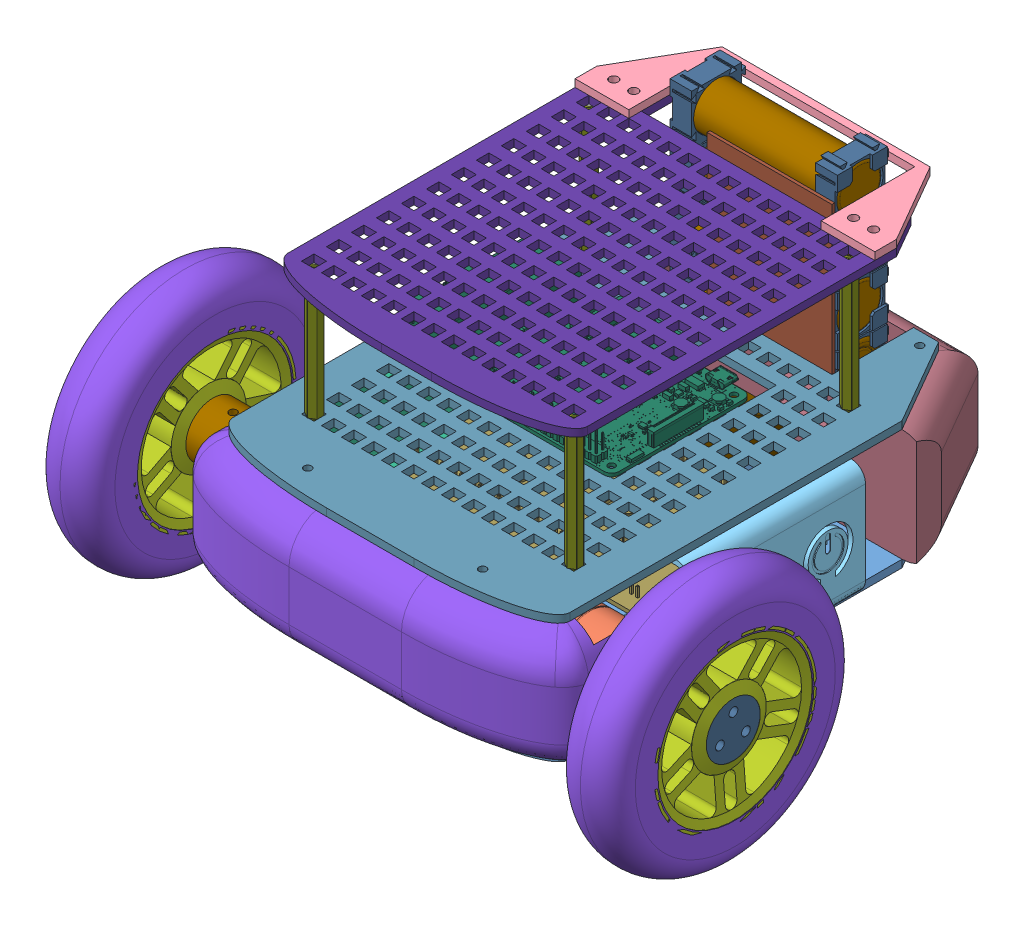
SolidWorks assembly EnsambleRobot, configuration Predeterminado. Lengths in mm.
Overall size (232.39 152.13 220.17).
59 component instances, 28 part files, 47 mates.
Components (placement in the parent):
- B00-1: B00 [Predeterminado] at (9.8412 177.5 6.4393) size (135.31 3.5 180.25)
- JA25-371-12V-1: JA25-371-12V [Predeterminado] at (-23.0941 197.7621 49.477) x (0 0 1) z (-1 0 0) size (25 25 76.39)
  - Gearbox-1: Gearbox [Predeterminado] at (16.9623 5.2379 20.5646) size (25 25 21)
  - hub-1: hub [Predeterminado] at (16.9623 5.2379 39.5646) x (0.985611 -0.169031 0) z (0 0 1) size (6.95 6.95 4.5)
  - Motor-1: Motor [Predeterminado] at (16.9623 5.2379 -9.9354) size (24.2 24.2 30.5)
  - Axis-1: Axis [Predeterminado] at (16.9623 5.2379 39.5646) x (0.853161 0.521648 0) z (0 0 1) size (4 4 14)
  - PCB-1: PCB [Predeterminado] at (16.9623 5.2379 -11.4354) x (-1 0 0) z (0 0 -1) size (23 23 4.73)
  - Magnet-1: Magnet [Predeterminado] at (16.9623 5.2379 -17.3254) x (-0.17817 -0.984 0) z (0 0 -1) size (14.2 14.2 15.5)
- JA25-371-12V-2: JA25-371-12V [Predeterminado] at (42.7766 208.2379 49.477) x (0 0 1) z (1 0 0) size (25 25 76.39)
  - Gearbox-1: Gearbox [Predeterminado] at (16.9623 5.2379 20.5646) size (25 25 21)
  - hub-1: hub [Predeterminado] at (16.9623 5.2379 39.5646) x (0.985611 -0.169031 0) z (0 0 1) size (6.95 6.95 4.5)
  - Motor-1: Motor [Predeterminado] at (16.9623 5.2379 -9.9354) size (24.2 24.2 30.5)
  - Axis-1: Axis [Predeterminado] at (16.9623 5.2379 39.5646) x (0.853161 0.521648 0) z (0 0 1) size (4 4 14)
  - PCB-1: PCB [Predeterminado] at (16.9623 5.2379 -11.4354) x (-1 0 0) z (0 0 -1) size (23 23 4.73)
  - Magnet-1: Magnet [Predeterminado] at (16.9623 5.2379 -17.3254) x (-0.17817 -0.984 0) z (0 0 -1) size (14.2 14.2 15.5)
- B01-1: B01 [Predeterminado] at (9.8412 180.5 76.4393) size (155.37 45.11 66.16)
- BatteryPack-1: BatteryPack [Predeterminado] at (-35.9513 260.8212 -115.5039) x (0 -1 0) z (0 0 1) size (86.68 67 25.44)
  - ELEB05-1: ELEB05 [По умолчанию] at (39.8212 13.291 48.4432) x (0.682904 0 -0.730508) z (0.730508 0 0.682904) size (18 65 18)
  - ELEB04-1: ELEB04 [Predeterminado] at (19.3212 20.991 48.4432) x (-1 0 0) z (0 0 1) size (21.5 8.7 21.5)
  - ELEB05-2: ELEB05 [По умолчанию] at (-1.1788 13.291 48.4432) x (0.778658 0 -0.627449) z (0.627449 0 0.778658) size (18 65 18)
  - ELEB05-3: ELEB05 [По умолчанию] at (-21.6788 78.291 48.4432) x (-0.837169 0 -0.546944) z (-0.546944 0 0.837169) size (18 65 18)
  - ELEB05-4: ELEB05 [По умолчанию] at (19.3212 78.291 48.4432) x (0.951676 0 -0.307103) z (-0.307103 0 -0.951676) size (18 65 18)
  - ELEB04-2: ELEB04 [Predeterminado] at (39.8212 70.591 48.4432) size (21.5 8.7 21.5)
  - ELEB04-3: ELEB04 [Predeterminado] at (-1.1788 70.591 48.4432) size (21.5 8.7 21.5)
  - ELEB04-4: ELEB04 [Predeterminado] at (19.3212 70.591 48.4432) size (21.5 8.7 21.5)
  - ELEB04-5: ELEB04 [Predeterminado] at (-21.6788 70.591 48.4432) size (21.5 8.7 21.5)
  - ELEB04-6: ELEB04 [Predeterminado] at (39.8212 20.991 48.4432) x (-1 0 0) z (0 0 1) size (21.5 8.7 21.5)
  - ELEB04-7: ELEB04 [Predeterminado] at (-21.6788 20.991 48.4432) x (-1 0 0) z (0 0 1) size (21.5 8.7 21.5)
  - ELEB04-8: ELEB04 [Predeterminado] at (-1.1788 20.991 48.4432) x (-1 0 0) z (0 0 1) size (21.5 8.7 21.5)
  - BMS-1: BMS [Default] at (8.3212 53.291 59.6432) x (-1 0 0) z (0 -1 0) size (60 1.2 50)
- stm30f4-1: stm30f4 [Default] at (-39.4234 195.5 39.7853) size (102.57 23 65.5)
- Back-1: Back [Predeterminado] at (9.8397 180.5 -71.2402) x (-1 0 0) z (0 0 -1) size (146.55 45 44.64)
- B001-1: B001 [Predeterminado] at (9.8412 225.5 6.4393) size (135.31 3.5 180.25)
- raspberryPi3B-1: raspberryPi3B [Detailed] at (7.0723 238.5 11.5542) x (-1 0 0) z (0 1 0) size (87.05 58.5 19.05)
- Spacer50mm-1: Spacer50mm [Varsayılan] at (-42.6588 278.5 66.2475) x (-0.866025 0 -0.5) z (-0.5 0 0.866025) size (5.71 56.2 5)
- Spacer50mm-2: Spacer50mm [Varsayılan] at (61.3412 278.5 -43.7587) x (-0.866025 0 -0.5) z (-0.5 0 0.866025) size (5.71 56.2 5)
- Spacer50mm-3: Spacer50mm [Varsayılan] at (61.3412 278.5 66.3559) x (-0.866025 0 -0.5) z (-0.5 0 0.866025) size (5.71 56.2 5)
- Spacer50mm-4: Spacer50mm [Varsayılan] at (-42.6588 278.5 -43.5) x (0 0 -1) z (-1 0 0) size (5.71 56.2 5)
- B002-1: B002 [Default] at (9.3412 278.5 6.4393) size (120.31 3.5 150.25)
- CasterJoint-1: CasterJoint [Default] at (30.1749 231.3692 -108.2134) x (-1 0 0) z (0 0 1) size (61 48.46 48.78)
  - C000-1: C000 [Default] at (20.3352 23.8692 48.4027) size (61 17 46)
  - C001-1: C001 [Default] at (20.3352 23.8692 48.4027) size (61 16.32 46)
  - BALL6MM-1: BALL6MM [Predeterminado] at (22.8352 26.8692 52.7329) size (6 6 6)
  - BALL40MM-1: BALL40MM [Default] at (20.3352 49.3191 48.4027) x (0.992761 -0.035378 0.11478) z (-0.109645 0.123176 0.986309) size (40 40 40)
  - BALL6MM-2: BALL6MM [Predeterminado] at (22.8352 26.8692 44.0726) size (6 6 6)
  - BALL6MM-3: BALL6MM [Predeterminado] at (15.3352 26.8692 48.4027) size (6 6 6)
- B03-1: B03 [Default] at (9.3412 281.5 -63.4728) size (120 3 40.5)
- B04-1: B04 [Default] at (52.713 199.7656 41.4393) x (-1 0 0) z (0 0 -1) size (78.74 45 70)
- B05-2: B05 [Default] at (-33.0305 199.7656 -28.5607) size (78.74 45 70)
- TuxsWheel100mm-1: TuxsWheel100mm [Default] at (-171.2257 152.4918 103.4572) x (0 0.055564 -0.998455) z (1 0 0) size (114.18 114.18 36.69)
  - B02-1: B02 [Default] at (39.7671 48.3733 64.9228) size (90.04 90.04 24)
  - B021-1: B021 [Default] at (39.7671 48.3733 64.9228) x (0.988174 0.153337 0) z (0 0 1) size (100.02 100.02 24.11)
  - Adapter1-1: Adapter1 [Default] at (39.7671 48.3733 72.3069) x (0.999683 0.025158 0) z (0 0 1) size (21.7 21.7 29.26)
  - Adapter2-1: Adapter2 [Default] at (39.7671 48.3733 65.8069) x (0.999683 0.025158 0) z (0 0 1) size (21.7 21.7 6.5)
- TuxsWheel100mm-2: TuxsWheel100mm [Default] at (190.9082 154.6267 26.6722) x (0 0 1) z (-1 0 0) size (114.18 114.18 36.69)
  - B02-1: B02 [Default] at (39.7671 48.3733 64.9228) size (90.04 90.04 24)
  - B021-1: B021 [Default] at (39.7671 48.3733 64.9228) x (0.988174 0.153337 0) z (0 0 1) size (100.02 100.02 24.11)
  - Adapter1-1: Adapter1 [Default] at (39.7671 48.3733 72.3069) x (0.999683 0.025158 0) z (0 0 1) size (21.7 21.7 29.26)
  - Adapter2-1: Adapter2 [Default] at (39.7671 48.3733 65.8069) x (0.999683 0.025158 0) z (0 0 1) size (21.7 21.7 6.5)
Mates (geometry in assembly coordinates):
- Coincident2: coincident anti-aligned: plane of B00-1 through (9.8412 180.5 6.4393) normal (0 1 0); plane of B01-1 through (9.8412 180.5 76.4393) normal (0 -1 0)
- Concentric1: concentric aligned: cylinder of JA25-371-12V-2/Axis-1 through (96.3412 203 66.4393) axis (-1 0 0) radius 2; cylinder of B01-1 through (87.6162 203 66.4393) axis (-1 0 0) radius 3.75
- Concentric2: concentric anti-aligned: cylinder of JA25-371-12V-2/Gearbox-1 through (63.3412 203 57.6893) axis (1 0 0) radius 1.5; cylinder of B01-1 through (87.6162 203 57.6893) axis (-1 0 0) radius 1.75
- Coincident5: coincident anti-aligned: plane of JA25-371-12V-2/Gearbox-1 through (84.3412 203 66.4393) normal (1 0 0); plane of B01-1 through (84.3412 27.4445 46.4393) normal (-1 0 0)
- Concentric3: concentric anti-aligned: cylinder of JA25-371-12V-1/Axis-1 through (-76.6588 203 66.4393) axis (1 0 0) radius 2; cylinder of B01-1 through (87.6162 203 66.4393) axis (-1 0 0) radius 3.75
- Coincident6: coincident anti-aligned: plane of JA25-371-12V-1/Gearbox-1 through (-64.6588 203 66.4393) normal (-1 0 0); plane of B01-1 through (-64.6588 27.4445 46.4393) normal (1 0 0)
- Concentric4: concentric aligned: cylinder of JA25-371-12V-1/Gearbox-1 through (-43.6588 203 57.6893) axis (-1 0 0) radius 1.5; cylinder of B01-1 through (87.6162 203 57.6893) axis (-1 0 0) radius 1.75
- Concentric5: concentric anti-aligned: cylinder of B00-1 through (-17.6588 177.5 51.4393) axis (0 1 0) radius 1.75; cylinder of B01-1 through (-17.6588 190.5 51.4393) axis (0 -1 0) radius 1.5
- Concentric6: concentric anti-aligned: cylinder of B00-1 through (37.3412 177.5 51.4393) axis (0 1 0) radius 1.75; cylinder of B01-1 through (37.3412 190.5 51.4393) axis (0 -1 0) radius 1.5
- Distance1: distance = 15 mm anti-aligned: plane of stm30f4-1 through (-39.4234 195.5 39.7853) normal (0 -1 0); plane of B00-1 through (9.8412 180.5 6.4393) normal (0 1 0)
- Coincident11: coincident anti-aligned: line of B00-1 through (57.3412 180.5 -83.5607) axis (-1 0 0); line of Back-1 through (-37.6618 180.5 -83.5607) axis (1 0 0)
- Coincident19: coincident anti-aligned: line of B00-1 through (77.3412 180.5 -48.9197) axis (-0.5 0 -0.866025); line of Back-1 through (57.3412 180.5 -83.5607) axis (0.5 0 0.866025)
- Coincident22: coincident anti-aligned: plane of Back-1 through (9.8397 225.5 -71.2402) normal (0 1 0); plane of B001-1 through (9.8412 225.5 6.4393) normal (0 -1 0)
- Coincident28: coincident aligned: plane of B00-1 through (-57.6588 180.5 -83.5607) normal (-1 0 0); plane of B001-1 through (-57.6588 228.5 -83.5607) normal (-1 0 0)
- Coincident29: coincident aligned: plane of B00-1 through (-57.6588 180.5 96.4393) normal (0 0 1); plane of B001-1 through (-57.6588 228.5 96.4393) normal (0 0 1)
- Distance11: distance = 10 mm anti-aligned: plane of raspberryPi3B-1 through (7.0723 238.5 11.5542) normal (0 -1 0); plane of B001-1 through (9.8412 228.5 6.4393) normal (0 1 0)
- Coincident47: coincident anti-aligned: plane of B001-1 through (9.8412 228.5 6.4393) normal (0 1 0); plane of Spacer50mm-4 through (-42.6588 228.5 -43.5) normal (0 -1 0)
- Coincident48: coincident anti-aligned: plane of B001-1 through (-45.1588 218.5 -46.0607) normal (1 0 0); plane of Spacer50mm-4 through (-45.1588 228.5 -42.0566) normal (-1 0 0)
- Coincident49: coincident anti-aligned: plane of B001-1 through (9.8412 228.5 6.4393) normal (0 1 0); plane of Spacer50mm-2 through (61.3412 228.5 -43.7587) normal (0 -1 0)
- Coincident50: coincident anti-aligned: plane of B001-1 through (63.8412 218.5 -46.0607) normal (-1 0 0); plane of Spacer50mm-2 through (63.8412 228.5 -45.2021) normal (1 0 0)
- Coincident52: coincident anti-aligned: plane of B001-1 through (9.8412 228.5 6.4393) normal (0 1 0); plane of Spacer50mm-1 through (-42.6588 228.5 66.2475) normal (0 -1 0)
- Coincident54: coincident aligned: plane of Spacer50mm-1 through (-45.1588 228.5 67.6909) normal (-1 0 0); plane of Spacer50mm-4 through (-45.1588 228.5 -42.0566) normal (-1 0 0)
- Coincident55: coincident anti-aligned: plane of B001-1 through (9.8412 228.5 6.4393) normal (0 1 0); plane of Spacer50mm-3 through (61.3412 228.5 66.3559) normal (0 -1 0)
- Coincident56: coincident anti-aligned: plane of B001-1 through (63.8412 218.5 63.9393) normal (-1 0 0); plane of Spacer50mm-3 through (63.8412 228.5 64.9125) normal (1 0 0)
- Coincident57: coincident anti-aligned: plane of Spacer50mm-3 through (61.3412 278.5 66.3559) normal (0 1 0); plane of B002-1 through (9.3412 278.5 6.4393) normal (0 -1 0)
- Coincident58: coincident aligned: plane of B001-1 through (-37.1588 218.5 63.9393) normal (0 0 1); plane of B002-1 through (-37.1588 278.5 63.9393) normal (0 0 1)
- Coincident59: coincident aligned: plane of B001-1 through (-37.1588 218.5 63.9393) normal (1 0 0); plane of B002-1 through (-37.1588 278.5 63.9393) normal (1 0 0)
- Coincident64: coincident anti-aligned: plane of Back-1 through (36.8397 207.5 -59.5607) normal (0 -1 0); plane of CasterJoint-1/C000-1 through (9.8397 207.5 -59.8107) normal (0 1 0)
- Parallel1: parallel anti-aligned: plane of Back-1 through (36.8397 207.5 -64.0607) normal (0 0 1); plane of CasterJoint-1/C000-1 through (36.8397 187.5 -63.0607) normal (0 0 -1)
- Concentric32: concentric aligned: cylinder of Back-1 through (-17.1603 189.5 -59.5607) axis (0 1 0) radius 1.75; cylinder of CasterJoint-1/C000-1 through (-17.1603 187.5 -59.5607) axis (0 1 0) radius 1.5
- Coincident66: coincident anti-aligned: plane of BatteryPack-1/ELEB04-6 through (-14.9603 209.5 -75.0107) normal (0 -1 0); plane of Back-1 through (36.8397 209.5 -59.5607) normal (0 1 0)
- Distance13: distance = 4 mm anti-aligned: plane of BatteryPack-1/ELEB04-6 through (-23.6603 221 -67.0607) normal (-1 0 0); plane of Back-1 through (-27.6603 125.9586 -83.5607) normal (1 0 0)
- Distance14: distance = 5 mm anti-aligned: plane of BatteryPack-1/ELEB04-2 through (34.6397 226.05 -78.5607) normal (0 0 -1); plane of Back-1 through (47.3397 125.9586 -83.5607) normal (0 0 1)
- Parallel3: parallel anti-aligned: plane of B002-1 through (9.3412 281.5 6.4393) normal (0 1 0); plane of B03-1 through (9.3412 281.5 -63.4728) normal (0 -1 0)
- Coincident73: coincident anti-aligned: plane of B002-1 through (9.3412 281.5 6.4393) normal (0 1 0); plane of B03-1 through (9.3412 281.5 -63.4728) normal (0 -1 0)
- Coincident74: coincident anti-aligned: line of B002-1 through (69.3412 278.5 -54.7043) axis (0 1 0); line of B03-1 through (69.3412 284.5 -54.7043) axis (0 -1 0)
- Coincident75: coincident aligned: plane of B002-1 through (69.3412 281.5 -68.5607) normal (1 0 0); plane of B03-1 through (69.3412 284.5 -54.7043) normal (1 0 0)
- Coincident79: coincident anti-aligned: plane of B00-1 through (9.8412 180.5 6.4393) normal (0 1 0); plane of B05-1 through (77.3412 180.5 -28.5607) normal (0 -1 0)
- Coincident80: coincident anti-aligned: line of B001-1 through (77.3412 225.5 83.9393) axis (0 0 -1); line of B05-1 through (77.3412 225.5 -28.5607) axis (0 0 1)
- Concentric33: concentric anti-aligned: cylinder of B00-1 through (69.8412 177.25 -18.5607) axis (0 1 0) radius 1.75; cylinder of B04-1 through (69.8412 225.501 -18.5607) axis (0 -1 0) radius 1.5
- Coincident81: coincident anti-aligned: plane of B00-1 through (9.8412 180.5 6.4393) normal (0 1 0); plane of B05-2 through (-57.6588 180.5 41.4393) normal (0 -1 0)
- Concentric43: concentric anti-aligned: cylinder of B00-1 through (-50.1588 177.25 -18.5607) axis (0 1 0) radius 1.75; cylinder of B05-2 through (-50.1588 225.501 -18.5607) axis (0 -1 0) radius 1.5
- Concentric44: concentric anti-aligned: cylinder of B00-1 through (-50.1588 177.25 31.4393) axis (0 1 0) radius 1.75; cylinder of B05-2 through (-50.1588 225.501 31.4393) axis (0 -1 0) radius 1.5
- Concentric45: concentric anti-aligned: cylinder of JA25-371-12V-1/Axis-1 through (-76.6588 203 66.4393) axis (1 0 0) radius 2; cylinder of TuxsWheel100mm-1/Adapter1-1 through (-89.6588 203 66.4393) axis (-1 0 0) radius 2.1
- Distance15: distance = 2 mm: plane of TuxsWheel100mm-1/Adapter1-1 through (-69.6588 203 66.4393) normal (1 0 0); line of B01-1 through (-67.6588 210.5 86.4393) axis (0 0 -1)
- Concentric46: concentric anti-aligned: cylinder of JA25-371-12V-2/Axis-1 through (96.3412 203 66.4393) axis (-1 0 0) radius 2; cylinder of TuxsWheel100mm-2/Adapter1-1 through (109.3412 203 66.4393) axis (1 0 0) radius 2.1
- Distance16: distance = 2 mm anti-aligned: plane of TuxsWheel100mm-2/Adapter1-1 through (89.3412 203 66.4393) normal (-1 0 0); plane of B01-1 through (87.3412 225.5 46.4393) normal (1 0 0)
